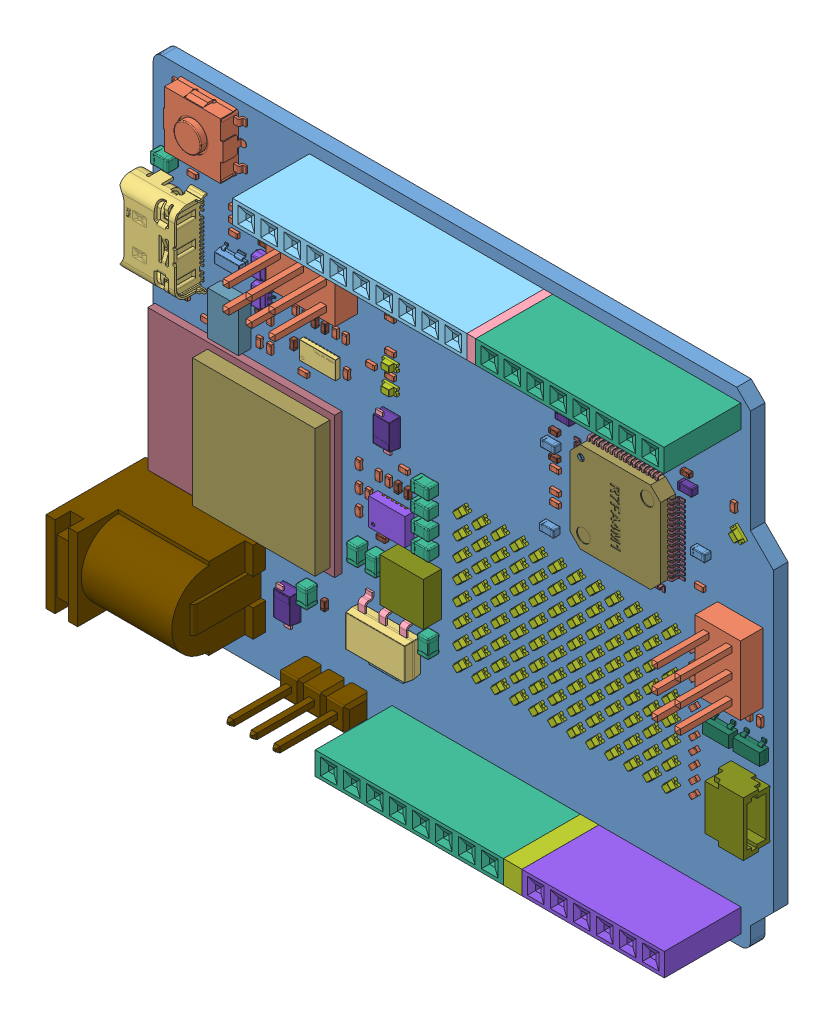
SolidWorks assembly Arduino UnoR4 Wifi PCB(ABX00087), configuration Standard. Lengths in mm. (continued)
Components (placement in the parent): (continued)
- PCB(ABX00087).step-1: PCB(ABX00087).step [Standard] at origin size (70.54 53.34 14.5) (continued)
  - U4.step-1: U4.step [Standard] at origin size (4 2 0.55) (continued)
    - IC_Texas_Instruments_TXB0108DQSR_eec.step-1: IC_Texas_Instruments_TXB0108DQSR_eec.step [Standard] at (13.565 34.6878 0.3) x (1 0 0) z (0 0 1) size (4 2 0.55) (continued)
      - Part16.step-5: Part16.step [Standard] at (5.331 -2.1143 -0.3) size (0.2 0.55 0.1)
      - Part16.step-6: Part16.step [Standard] at (5.731 -2.1143 -0.3) size (0.2 0.55 0.1)
      - Part16.step-7: Part16.step [Standard] at (6.131 -2.1143 -0.3) size (0.2 0.55 0.1)
      - Part16.step-8: Part16.step [Standard] at (6.531 -2.1143 -0.3) size (0.2 0.55 0.1)
      - Part16.step-9: Part16.step [Standard] at (6.931 -2.1143 -0.3) size (0.2 0.55 0.1)
      - Part16_MIR.step-1: Part16_MIR.step [Standard] at (3.731 -0.6643 -0.3) x (1 0 0) z (0 0 -1) size (0.2 0.55 0.1)
      - Part16_MIR.step-2: Part16_MIR.step [Standard] at (3.331 -0.6643 -0.3) x (1 0 0) z (0 0 -1) size (0.2 0.55 0.1)
      - Part16_MIR1.step-1: Part16_MIR1.step [Standard] at (4.131 -0.6643 -0.3) x (1 0 0) z (0 0 -1) size (0.2 0.55 0.1)
      - Part16_MIR1.step-2: Part16_MIR1.step [Standard] at (4.531 -0.6643 -0.3) x (1 0 0) z (0 0 -1) size (0.2 0.55 0.1)
      - Part16_MIR1.step-3: Part16_MIR1.step [Standard] at (4.931 -0.6643 -0.3) x (1 0 0) z (0 0 -1) size (0.2 0.55 0.1)
      - Part16_MIR1.step-4: Part16_MIR1.step [Standard] at (5.331 -0.6643 -0.3) x (1 0 0) z (0 0 -1) size (0.2 0.55 0.1)
      - Part16_MIR1.step-5: Part16_MIR1.step [Standard] at (5.731 -0.6643 -0.3) x (1 0 0) z (0 0 -1) size (0.2 0.55 0.1)
      - Part16_MIR1.step-6: Part16_MIR1.step [Standard] at (6.131 -0.6643 -0.3) x (1 0 0) z (0 0 -1) size (0.2 0.55 0.1)
      - Part16_MIR1.step-7: Part16_MIR1.step [Standard] at (6.531 -0.6643 -0.3) x (1 0 0) z (0 0 -1) size (0.2 0.55 0.1)
      - Part16_MIR1.step-8: Part16_MIR1.step [Standard] at (6.931 -0.6643 -0.3) x (1 0 0) z (0 0 -1) size (0.2 0.55 0.1)
      - Part16 - Copy.step-1: Part16 - Copy.step [Standard] at (3.331 -2.0643 -0.3) size (0.2 0.65 0.1)
  - C24.step-1: C24.step [Standard] at origin size (0.5 1 0.5)
    - CAP-0402.step-1: CAP-0402.step [Standard] at (18.146 36.576 0) x (0 -1 0) z (0 0 1) size (1 0.5 0.5)
  - C25.step-1: C25.step [Standard] at origin size (0.5 1 0.5)
    - CAP-0402.step-1: CAP-0402.step [Standard] at (19.246 36.576 0) x (0 -1 0) z (0 0 1) size (1 0.5 0.5)
  - C26.step-1: C26.step [Standard] at origin size (0.5 1 0.5)
    - CAP-0402.step-1: CAP-0402.step [Standard] at (15.796 33.276 0) x (0 1 0) z (0 0 1) size (1 0.5 0.5)
  - U3.step-1: U3.step [Standard] at origin size (4 3 1)
    - 6430905744.step-1: 6430905744.step [Standard] at (26.825 22.1 0) x (0 1 0) z (0 0 1) size (3 4 1)
      - Body-3.step-1: Body-3.step [Standard] at (-1.5 -2 0) size (3 4 1)
        - Open CASCADE STEP translator 6.8 36.2.1.step-1: Open CASCADE STEP translator 6.8 36.2.1.step [Standard] at origin size (3 4 1)
      - Pin_Shape.step-1: Pin_Shape.step [Standard] at (-1.5 -1.3675 0) size (0.4 0.23 0.2)
        - Open CASCADE STEP translator 6.8 36.4.1.step-1: Open CASCADE STEP translator 6.8 36.4.1.step [Standard] at origin size (0.4 0.23 0.2)
      - Pin_Shape.step-2: Pin_Shape.step [Standard] at (1.5 1.3675 0) x (-1 0 0) z (0 0 1) size (0.4 0.23 0.2)
        - Open CASCADE STEP translator 6.8 36.4.1.step-1: Open CASCADE STEP translator 6.8 36.4.1.step [Standard] at origin size (0.4 0.23 0.2)
      - Pin_Shape.step-3: Pin_Shape.step [Standard] at (-1.5 -0.8675 0) size (0.4 0.23 0.2)
        - Open CASCADE STEP translator 6.8 36.4.1.step-1: Open CASCADE STEP translator 6.8 36.4.1.step [Standard] at origin size (0.4 0.23 0.2)
      - Pin_Shape.step-4: Pin_Shape.step [Standard] at (1.5 0.8675 0) x (-1 0 0) z (0 0 1) size (0.4 0.23 0.2)
        - Open CASCADE STEP translator 6.8 36.4.1.step-1: Open CASCADE STEP translator 6.8 36.4.1.step [Standard] at origin size (0.4 0.23 0.2)
      - Pin_Shape.step-5: Pin_Shape.step [Standard] at (-1.5 -0.3675 0) size (0.4 0.23 0.2)
        - Open CASCADE STEP translator 6.8 36.4.1.step-1: Open CASCADE STEP translator 6.8 36.4.1.step [Standard] at origin size (0.4 0.23 0.2)
      - Pin_Shape.step-6: Pin_Shape.step [Standard] at (1.5 0.3675 0) x (-1 0 0) z (0 0 1) size (0.4 0.23 0.2)
        - Open CASCADE STEP translator 6.8 36.4.1.step-1: Open CASCADE STEP translator 6.8 36.4.1.step [Standard] at origin size (0.4 0.23 0.2)
      - Pin_Shape.step-7: Pin_Shape.step [Standard] at (-1.5 0.1325 0) size (0.4 0.23 0.2)
        - Open CASCADE STEP translator 6.8 36.4.1.step-1: Open CASCADE STEP translator 6.8 36.4.1.step [Standard] at origin size (0.4 0.23 0.2)
      - Pin_Shape.step-8: Pin_Shape.step [Standard] at (1.5 -0.1325 0) x (-1 0 0) z (0 0 1) size (0.4 0.23 0.2)
        - Open CASCADE STEP translator 6.8 36.4.1.step-1: Open CASCADE STEP translator 6.8 36.4.1.step [Standard] at origin size (0.4 0.23 0.2)
      - Pin_Shape.step-9: Pin_Shape.step [Standard] at (-1.5 0.6325 0) size (0.4 0.23 0.2)
        - Open CASCADE STEP translator 6.8 36.4.1.step-1: Open CASCADE STEP translator 6.8 36.4.1.step [Standard] at origin size (0.4 0.23 0.2)
      - Pin_Shape.step-10: Pin_Shape.step [Standard] at (1.5 -0.6325 0) x (-1 0 0) z (0 0 1) size (0.4 0.23 0.2)
        - Open CASCADE STEP translator 6.8 36.4.1.step-1: Open CASCADE STEP translator 6.8 36.4.1.step [Standard] at origin size (0.4 0.23 0.2)
      - Pin_Shape.step-11: Pin_Shape.step [Standard] at (-1.5 1.1325 0) size (0.4 0.23 0.2)
        - Open CASCADE STEP translator 6.8 36.4.1.step-1: Open CASCADE STEP translator 6.8 36.4.1.step [Standard] at origin size (0.4 0.23 0.2)
      - Pin_Shape.step-12: Pin_Shape.step [Standard] at (1.5 -1.1325 0) x (-1 0 0) z (0 0 1) size (0.4 0.23 0.2)
        - Open CASCADE STEP translator 6.8 36.4.1.step-1: Open CASCADE STEP translator 6.8 36.4.1.step [Standard] at origin size (0.4 0.23 0.2)
      - Open CASCADE STEP translator 6.8 36.1.step-1: Open CASCADE STEP translator 6.8 36.1.step [Standard] at (-1.5 -2 0) size (0.38 0.38 0)
      - Thermal_Shape.step-1: Thermal_Shape.step [Standard] at (-0.8375 -1.6375 -0.001) size (1.68 3.28 0)
  - U1.step-1: U1.step [Standard] at origin size (12.2 12.2 1.68)
    - RA4M1 v4.step-1: RA4M1 v4.step [Standard] at (40.7498 25.853 0) size (12.2 12.2 1.67)
      - Designator1.step-1: Designator1.step [Standard] at origin size (12.2 12.2 1.67)
        - 6422462560.step-1: 6422462560.step [Standard] at (12 10 0) size (12.2 12.2 1.65)
          - Body-4.step-1: Body-4.step [Standard] at (-5 -5 0) size (10 10 1.65)
            - Open CASCADE STEP translator 6.8 23.1.1.step-1: Open CASCADE STEP translator 6.8 23.1.1.step [Standard] at origin size (10 10 1.65)
          - Leader-2.step-1: Leader-2.step [Standard] at (-5 -3.75 0) x (-1 0 0) z (0 0 1) size (1.1 0.27 0.88)
          - Leader-2.step-2: Leader-2.step [Standard] at (-3.75 5 0) x (0 1 0) z (0 0 1) size (1.1 0.27 0.88)
          - Leader-2.step-3: Leader-2.step [Standard] at (5 -3.75 0) size (1.1 0.27 0.88)
          - Leader-2.step-4: Leader-2.step [Standard] at (-3.75 -5 0) x (0 -1 0) z (0 0 1) size (1.1 0.27 0.88)
          - Leader-2.step-5: Leader-2.step [Standard] at (-5 -3.25 0) x (-1 0 0) z (0 0 1) size (1.1 0.27 0.88)
          - Leader-2.step-6: Leader-2.step [Standard] at (-3.25 5 0) x (0 1 0) z (0 0 1) size (1.1 0.27 0.88)
          - Leader-2.step-7: Leader-2.step [Standard] at (5 -3.25 0) size (1.1 0.27 0.88)
          - Leader-2.step-8: Leader-2.step [Standard] at (-3.25 -5 0) x (0 -1 0) z (0 0 1) size (1.1 0.27 0.88)
          - Leader-2.step-9: Leader-2.step [Standard] at (-5 -2.75 0) x (-1 0 0) z (0 0 1) size (1.1 0.27 0.88)
          - Leader-2.step-10: Leader-2.step [Standard] at (-2.75 5 0) x (0 1 0) z (0 0 1) size (1.1 0.27 0.88)
          - Leader-2.step-11: Leader-2.step [Standard] at (5 -2.75 0) size (1.1 0.27 0.88)
          - Leader-2.step-12: Leader-2.step [Standard] at (-2.75 -5 0) x (0 -1 0) z (0 0 1) size (1.1 0.27 0.88)
          - Leader-2.step-13: Leader-2.step [Standard] at (-5 -2.25 0) x (-1 0 0) z (0 0 1) size (1.1 0.27 0.88)
          - Leader-2.step-14: Leader-2.step [Standard] at (-2.25 5 0) x (0 1 0) z (0 0 1) size (1.1 0.27 0.88)
          - Leader-2.step-15: Leader-2.step [Standard] at (5 -2.25 0) size (1.1 0.27 0.88)
          - Leader-2.step-16: Leader-2.step [Standard] at (-2.25 -5 0) x (0 -1 0) z (0 0 1) size (1.1 0.27 0.88)
          - Leader-2.step-17: Leader-2.step [Standard] at (-5 -1.75 0) x (-1 0 0) z (0 0 1) size (1.1 0.27 0.88)
          - Leader-2.step-18: Leader-2.step [Standard] at (-1.75 5 0) x (0 1 0) z (0 0 1) size (1.1 0.27 0.88)
          - Leader-2.step-19: Leader-2.step [Standard] at (5 -1.75 0) size (1.1 0.27 0.88)
          - Leader-2.step-20: Leader-2.step [Standard] at (-1.75 -5 0) x (0 -1 0) z (0 0 1) size (1.1 0.27 0.88)
          - Leader-2.step-21: Leader-2.step [Standard] at (-5 -1.25 0) x (-1 0 0) z (0 0 1) size (1.1 0.27 0.88)
          - Leader-2.step-22: Leader-2.step [Standard] at (-1.25 5 0) x (0 1 0) z (0 0 1) size (1.1 0.27 0.88)
          - Leader-2.step-23: Leader-2.step [Standard] at (5 -1.25 0) size (1.1 0.27 0.88)
          - Leader-2.step-24: Leader-2.step [Standard] at (-1.25 -5 0) x (0 -1 0) z (0 0 1) size (1.1 0.27 0.88)
          - Leader-2.step-25: Leader-2.step [Standard] at (-5 -0.75 0) x (-1 0 0) z (0 0 1) size (1.1 0.27 0.88)
          - Leader-2.step-26: Leader-2.step [Standard] at (-0.75 5 0) x (0 1 0) z (0 0 1) size (1.1 0.27 0.88)
          - Leader-2.step-27: Leader-2.step [Standard] at (5 -0.75 0) size (1.1 0.27 0.88)
          - Leader-2.step-28: Leader-2.step [Standard] at (-0.75 -5 0) x (0 -1 0) z (0 0 1) size (1.1 0.27 0.88)
          - Leader-2.step-29: Leader-2.step [Standard] at (-5 -0.25 0) x (-1 0 0) z (0 0 1) size (1.1 0.27 0.88)
          - Leader-2.step-30: Leader-2.step [Standard] at (-0.25 5 0) x (0 1 0) z (0 0 1) size (1.1 0.27 0.88)
          - Leader-2.step-31: Leader-2.step [Standard] at (5 -0.25 0) size (1.1 0.27 0.88)
          - Leader-2.step-32: Leader-2.step [Standard] at (-0.25 -5 0) x (0 -1 0) z (0 0 1) size (1.1 0.27 0.88)
          - Leader-2.step-33: Leader-2.step [Standard] at (-5 0.25 0) x (-1 0 0) z (0 0 1) size (1.1 0.27 0.88)
          - Leader-2.step-34: Leader-2.step [Standard] at (0.25 5 0) x (0 1 0) z (0 0 1) size (1.1 0.27 0.88)
          - Leader-2.step-35: Leader-2.step [Standard] at (5 0.25 0) size (1.1 0.27 0.88)
          - Leader-2.step-36: Leader-2.step [Standard] at (0.25 -5 0) x (0 -1 0) z (0 0 1) size (1.1 0.27 0.88)
          - Leader-2.step-37: Leader-2.step [Standard] at (-5 0.75 0) x (-1 0 0) z (0 0 1) size (1.1 0.27 0.88)
          - Leader-2.step-38: Leader-2.step [Standard] at (0.75 5 0) x (0 1 0) z (0 0 1) size (1.1 0.27 0.88)
          - Leader-2.step-39: Leader-2.step [Standard] at (5 0.75 0) size (1.1 0.27 0.88)
          - Leader-2.step-40: Leader-2.step [Standard] at (0.75 -5 0) x (0 -1 0) z (0 0 1) size (1.1 0.27 0.88)
          - Leader-2.step-41: Leader-2.step [Standard] at (-5 1.25 0) x (-1 0 0) z (0 0 1) size (1.1 0.27 0.88)
          - Leader-2.step-42: Leader-2.step [Standard] at (1.25 5 0) x (0 1 0) z (0 0 1) size (1.1 0.27 0.88)
          - Leader-2.step-43: Leader-2.step [Standard] at (5 1.25 0) size (1.1 0.27 0.88)
          - Leader-2.step-44: Leader-2.step [Standard] at (1.25 -5 0) x (0 -1 0) z (0 0 1) size (1.1 0.27 0.88)
          - Leader-2.step-45: Leader-2.step [Standard] at (-5 1.75 0) x (-1 0 0) z (0 0 1) size (1.1 0.27 0.88)
          - Leader-2.step-46: Leader-2.step [Standard] at (1.75 5 0) x (0 1 0) z (0 0 1) size (1.1 0.27 0.88)
          - Leader-2.step-47: Leader-2.step [Standard] at (5 1.75 0) size (1.1 0.27 0.88)
          - Leader-2.step-48: Leader-2.step [Standard] at (1.75 -5 0) x (0 -1 0) z (0 0 1) size (1.1 0.27 0.88)
          - Leader-2.step-49: Leader-2.step [Standard] at (-5 2.25 0) x (-1 0 0) z (0 0 1) size (1.1 0.27 0.88)
          - Leader-2.step-50: Leader-2.step [Standard] at (2.25 5 0) x (0 1 0) z (0 0 1) size (1.1 0.27 0.88)
          - Leader-2.step-51: Leader-2.step [Standard] at (5 2.25 0) size (1.1 0.27 0.88)
          - Leader-2.step-52: Leader-2.step [Standard] at (2.25 -5 0) x (0 -1 0) z (0 0 1) size (1.1 0.27 0.88)
          - Leader-2.step-53: Leader-2.step [Standard] at (-5 2.75 0) x (-1 0 0) z (0 0 1) size (1.1 0.27 0.88)
          - Leader-2.step-54: Leader-2.step [Standard] at (2.75 5 0) x (0 1 0) z (0 0 1) size (1.1 0.27 0.88)
          - Leader-2.step-55: Leader-2.step [Standard] at (5 2.75 0) size (1.1 0.27 0.88)
          - Leader-2.step-56: Leader-2.step [Standard] at (2.75 -5 0) x (0 -1 0) z (0 0 1) size (1.1 0.27 0.88)
          - Leader-2.step-57: Leader-2.step [Standard] at (-5 3.25 0) x (-1 0 0) z (0 0 1) size (1.1 0.27 0.88)
          - Leader-2.step-58: Leader-2.step [Standard] at (3.25 5 0) x (0 1 0) z (0 0 1) size (1.1 0.27 0.88)
          - Leader-2.step-59: Leader-2.step [Standard] at (5 3.25 0) size (1.1 0.27 0.88)
          - Leader-2.step-60: Leader-2.step [Standard] at (3.25 -5 0) x (0 -1 0) z (0 0 1) size (1.1 0.27 0.88)
          - Leader-2.step-61: Leader-2.step [Standard] at (-5 3.75 0) x (-1 0 0) z (0 0 1) size (1.1 0.27 0.88)
          - Leader-2.step-62: Leader-2.step [Standard] at (3.75 5 0) x (0 1 0) z (0 0 1) size (1.1 0.27 0.88)
          - Leader-2.step-63: Leader-2.step [Standard] at (5 3.75 0) size (1.1 0.27 0.88)
          - Leader-2.step-64: Leader-2.step [Standard] at (3.75 -5 0) x (0 -1 0) z (0 0 1) size (1.1 0.27 0.88)
        - 7219473552.step-1: 7219473552.step [Standard] at (8.2001 13.7999 0.25) size (0.7 0.7 1.42)
          - Extruded-3.step-1: Extruded-3.step [Standard] at origin size (0.7 0.7 1.42)
    - 6360838992.step-1: 6360838992.step [Standard] at (48.9498 39.6529 0.25) size (0.7 0.71 1.43)
      - Extruded-4.step-1: Extruded-4.step [Standard] at origin size (0.7 0.71 1.43)
  - R23.step-1: R23.step [Standard] at origin size (1 0.5 0.34)
    - RES-0402.step-1: RES-0402.step [Standard] at (26.416 35.433 0) size (1 0.5 0.34)
  - R40.step-1: R40.step [Standard] at origin size (0.5 1 0.34)
    - RES-0402.step-1: RES-0402.step [Standard] at (25.125 25.3 0) x (0 -1 0) z (0 0 1) size (1 0.5 0.34)
  - R38.step-1: R38.step [Standard] at origin size (0.5 1 0.34)
    - RES-0402.step-1: RES-0402.step [Standard] at (26.225 25.3 0) x (0 -1 0) z (0 0 1) size (1 0.5 0.34)
  - R36.step-1: R36.step [Standard] at origin size (1 0.5 0.34)
    - RES-0402.step-1: RES-0402.step [Standard] at (27.95 27.235 0) x (-1 0 0) z (0 0 1) size (1 0.5 0.34)
  - R44.step-1: R44.step [Standard] at origin size (0.5 1 0.34)
    - RES-0402.step-1: RES-0402.step [Standard] at (22.925 23 0) x (0 1 0) z (0 0 1) size (1 0.5 0.34)
  - R43.step-1: R43.step [Standard] at origin size (0.5 1 0.34)
    - RES-0402.step-1: RES-0402.step [Standard] at (22.925 25.3 0) x (0 -1 0) z (0 0 1) size (1 0.5 0.34)
  - R7.step-1: R7.step [Standard] at origin size (1 0.5 0.34)
    - RES-0402.step-1: RES-0402.step [Standard] at (60.646 32.376 0) x (-1 0 0) z (0 0 1) size (1 0.5 0.34)
  - R1.step-1: R1.step [Standard] at origin size (0.5 1 0.34)
    - RES-0402.step-1: RES-0402.step [Standard] at (13.125 34.231 0) x (0 1 0) z (0 0 1) size (1 0.5 0.34)
  - L3.step-1: L3.step [Standard] at origin size (4.8 4.8 2)
    - 6431045296.step-1: 6431045296.step [Standard] at (29.5083 17.2482 0.05) size (4.8 4.8 2)
      - Extruded-5.step-1: Extruded-5.step [Standard] at origin size (4.8 4.8 2)
  - L2.step-1: L2.step [Standard] at origin size (1.6 0.8 0.8)
    - FER-0603.step-1: FER-0603.step [Standard] at (59.5098 41.428 0) x (1 0 0) z (0 0 1) size (1.6 0.8 0.8)
  - L1.step-1: L1.step [Standard] at origin size (1.6 0.8 0.8)
    - FER-0603.step-1: FER-0603.step [Standard] at (45.9897 41.428 0) x (1 0 0) z (0 0 1) size (1.6 0.8 0.8)
  - C16.step-1: C16.step [Standard] at origin size (2 1.25 1.25)
    - CAP-0805.step-1: CAP-0805.step [Standard] at (30.6599 23.2481 0) x (-1 0 0) z (0 0 1) size (2 1.25 1.25)
  - C11.step-1: C11.step [Standard] at origin size (0.5 1 0.5)
    - CAP-0402.step-1: CAP-0402.step [Standard] at (19.19 9.991 0) x (0 1 0) z (0 0 1) size (1 0.5 0.5)
  - C19.step-1: C19.step [Standard] at origin size (1.25 2 1.25)
    - CAP-0805.step-1: CAP-0805.step [Standard] at (25.2157 17.2529 0) x (0 -1 0) z (0 0 1) size (2 1.25 1.25)
  - C14.step-1: C14.step [Standard] at origin size (0.5 1 0.5)
    - CAP-0402.step-1: CAP-0402.step [Standard] at (27.325 25.3 0) x (0 1 0) z (0 0 1) size (1 0.5 0.5)
  - C15.step-1: C15.step [Standard] at origin size (2 1.25 1.25)
    - CAP-0805.step-1: CAP-0805.step [Standard] at (30.6599 21.2981 0) x (-1 0 0) z (0 0 1) size (2 1.25 1.25)
  - C13.step-1: C13.step [Standard] at origin size (1.25 2 1.25)
    - CAP-0805.step-1: CAP-0805.step [Standard] at (23.199 17.2531 0) x (0 1 0) z (0 0 1) size (2 1.25 1.25)
  - C12.step-1: C12.step [Standard] at origin size (1 0.5 0.5)
    - CAP-0402.step-1: CAP-0402.step [Standard] at (25.6 19.6 0) size (1 0.5 0.5)
  - C20.step-1: C20.step [Standard] at origin size (0.5 1 0.5)
    - CAP-0402.step-1: CAP-0402.step [Standard] at (28.425 25.3 0) x (0 1 0) z (0 0 1) size (1 0.5 0.5)
  - C9.step-1: C9.step [Standard] at origin size (1.6 0.8 0.8)
    - CAP-0603.step-1: CAP-0603.step [Standard] at (44.3498 37.953 0) size (1.6 0.8 0.8)
  - C8.step-1: C8.step [Standard] at origin size (1 0.5 0.5)
    - CAP-0402.step-1: CAP-0402.step [Standard] at (44.6495 39.306 0) size (1 0.5 0.5)
  - C6.step-1: C6.step [Standard] at origin size (1 0.5 0.5)
    - CAP-0402.step-1: CAP-0402.step [Standard] at (59.2348 42.628 0) size (1 0.5 0.5)
  - C3.step-1: C3.step [Standard] at origin size (1 0.5 0.5)
    - CAP-0402.step-1: CAP-0402.step [Standard] at (44.646 36.776 0) size (1 0.5 0.5)
  - C2.step-1: C2.step [Standard] at origin size (1.6 0.8 0.8)
    - CAP-0603.step-1: CAP-0603.step [Standard] at (60.946 35.876 0) x (-1 0 0) z (0 0 1) size (1.6 0.8 0.8)
  - R51.step-1: R51.step [Standard] at origin size (1 0.5 0.34)
    - RES-0402.step-1: RES-0402.step [Standard] at (9.125 41.6599 0) x (-1 0 0) z (0 0 1) size (1 0.5 0.34)
  - R50.step-1: R50.step [Standard] at origin size (1 0.5 0.34)
    - RES-0402.step-1: RES-0402.step [Standard] at (9.125 40.466 0) x (-1 0 0) z (0 0 1) size (1 0.5 0.34)
  - R15.step-1: R15.step [Standard] at origin size (1 0.5 0.34)
    - RES-0402.step-1: RES-0402.step [Standard] at (44.646 33.476 0) size (1 0.5 0.34)
  - R18.step-1: R18.step [Standard] at origin size (0.5 1 0.34)
    - RES-0402.step-1: RES-0402.step [Standard] at (11.925 31.466 0) x (0 -1 0) z (0 0 1) size (1 0.5 0.34)
  - R24.step-1: R24.step [Standard] at origin size (0.5 1 0.34)
    - RES-0402.step-1: RES-0402.step [Standard] at (64.3844 41.9405 0) x (0 -1 0) z (0 0 1) size (1 0.5 0.34)
  - R19.step-1: R19.step [Standard] at origin size (1 0.5 0.34)
    - RES-0402.step-1: RES-0402.step [Standard] at (44.646 32.376 0) size (1 0.5 0.34)
  - R49.step-1: R49.step [Standard] at origin size (0.5 1 0.34)
    - RES-0402.step-1: RES-0402.step [Standard] at (21.596 33.276 0) x (0 1 0) z (0 0 1) size (1 0.5 0.34)
  - R25.step-1: R25.step [Standard] at origin size (1 0.5 0.34)
    - RES-0402.step-1: RES-0402.step [Standard] at (26.416 43.307 0) size (1 0.5 0.34)
  - DL3.step-1: DL3.step [Standard] at origin size (1.7 1.7 0.8)
    - HSMx-190.step-1: HSMx-190.step [Standard] at (64.897 39.5529 0) x (0.707107 -0.707107 0) z (0 0 1) size (1.6 0.8 0.8)
  - C21.step-1: C21.step [Standard] at origin size (2 1.25 1.25)
    - CAP-0805.step-1: CAP-0805.step [Standard] at (1.8498 44.1531 0) size (2 1.25 1.25)
  - R22.step-1: R22.step [Standard] at origin size (1 0.5 0.34)
    - RES-0402.step-1: RES-0402.step [Standard] at (26.416 37.719 0) size (1 0.5 0.34)
  - DL2.step-1: DL2.step [Standard] at origin size (1.6 0.8 0.8)
    - HSMx-190.step-1: HSMx-190.step [Standard] at (26.416 34.29 0) x (1 0 0) z (0 0 1) size (1.6 0.8 0.8)
  - DL1.step-1: DL1.step [Standard] at origin size (1.6 0.8 0.8)
    - HSMx-190.step-1: HSMx-190.step [Standard] at (26.416 36.576 0) x (1 0 0) z (0 0 1) size (1.6 0.8 0.8)
  - DL4.step-1: DL4.step [Standard] at origin size (1.6 0.8 0.8)
    - HSMx-190.step-1: HSMx-190.step [Standard] at (26.416 42.164 0) x (1 0 0) z (0 0 1) size (1.6 0.8 0.8)
  - R17.step-1: R17.step [Standard] at origin size (0.5 1 0.34)
    - RES-0402.step-1: RES-0402.step [Standard] at (13.125 31.4599 0) x (0 -1 0) z (0 0 1) size (1 0.5 0.34)
  - C7.step-1: C7.step [Standard] at origin size (1 0.5 0.5)
    - CAP-0402.step-1: CAP-0402.step [Standard] at (46.2648 42.628 0) size (1 0.5 0.5)
  - J5.step-1: J5.step [Standard] at origin size (14.4 9.4 14.5)
    - pj-102ah.step-1: pj-102ah.step [Standard] at (-1.96 8.3559 5.3937) x (-1 0 0) z (0 1 0) size (14.4 14.5 9.4)
  - D2.step-1: D2.step [Standard] at origin size (2.01 3.7 1.2)
    - SOD123FL.step-1: SOD123FL.step [Standard] at (28.396 26.476 0) x (0 1 0) z (0 0 1) size (3.7 2 1.2)
      - 8279795424.step-1: 8279795424.step [Standard] at (4 2 0) size (3.7 2 1.2)
        - Body-2.step-1: Body-2.step [Standard] at (-1.5 -1 0) size (3 2 1.2)
          - Open CASCADE STEP translator 7.5 15.1.1.step-1: Open CASCADE STEP translator 7.5 15.1.1.step [Standard] at origin size (3 2 1.2)
        - Lead.step-1: Lead.step [Standard] at (-1.85 -0.425 0) size (1.65 0.75 1.01)
        - Lead.step-2: Lead.step [Standard] at (1.85 0.425 0) x (-1 0 0) z (0 0 1) size (1.65 0.75 1.01)
  - D3.step-1: D3.step [Standard] at origin size (2.9 2.31 1)
    - PRTR5V0U2X.step-1: PRTR5V0U2X.step [Standard] at (9.125 37.866 0) x (-1 0 0) z (0 0 1) size (2.9 2.31 1)
  - J3.step-1: J3.step [Standard] at origin size (5.04 7.62 11.5)
    - 2x3 Header.step-1: 2x3 Header.step [Standard] at (67.4371 24.1301 0) x (-1 0 0) z (0 1 0) size (5.04 11.5 7.62)
  - PB1.step-1: PB1.step [Standard] at origin size (8.2 6.5 2.66)
    - TETactileSwitch1571636.step-1: TETactileSwitch1571636.step [Standard] at (6.3501 49.4031 2) size (8.2 6.5 2.66)
  - R39.step-1: R39.step [Standard] at origin size (1 0.5 0.34)
    - RES-0402.step-1: RES-0402.step [Standard] at (4.5498 43.853 0) x (-1 0 0) z (0 0 1) size (1 0.5 0.34)
  - J1.step-1: J1.step [Standard] at origin size (6.8 9.54 3.62)
    - CX90B-16P_CL0480-0755-0-00_3DDrawing_STEP_CX90B-16P_3D_48007525000_3D_STP.step-1: CX90B-16P_CL0480-0755-0-00_3DDrawing_STEP_CX90B-16P_3D_48007525000_3D_STP.step [Standard] at (3.8875 37.866 0.31) x (0 -1 0) z (0 0 1) size (9.54 6.8 3.62)
      - CX90B-16P_3D.step-1: CX90B-16P_3D.step [Standard] at (0.25 -4.65 1.28) x (1 0 0) z (0 -1 0) size (9.54 3.62 6.8)
  - JDIGITAL.step-1: JDIGITAL.step [Standard] at origin size (47.7 2.54 11.7)
    - 6431046176.step-1: 6431046176.step [Standard] at (43.6689 50.7997 0) size (0.99 2.54 8.5)
      - Extruded-6.step-1: Extruded-6.step [Standard] at origin size (0.99 2.54 8.5)
    - Header_Fem_1X10_digikey.step-1: Header_Fem_1X10_digikey.step [Standard] at (30.226 50.8 0) x (-1 0 0) z (0 1 0) size (25.9 11.7 2.54)
    - Header _Fem_1X8.step-1: Header _Fem_1X8.step [Standard] at (54.57 50.8 0) x (-1 0 0) z (0 1 0) size (20.82 11.7 2.54)
  - JANALOG.step-1: JANALOG.step [Standard] at origin size (38.6 2.54 11.7)
    - 6431040416.step-1: 6431040416.step [Standard] at (48.2497 2.5405 0) size (2.04 2.54 8.5)
      - Extruded-7.step-1: Extruded-7.step [Standard] at origin size (2.04 2.54 8.5)
    - Header _Fem_1X8.step-1: Header _Fem_1X8.step [Standard] at (36.82 2.54 0) x (1 0 0) z (0 -1 0) size (20.82 11.7 2.54)
    - Header_Fem_1X6_digikey.step-1: Header_Fem_1X6_digikey.step [Standard] at (57.14 2.54 0) x (1 0 0) z (0 -1 0) size (15.74 11.7 2.54)
